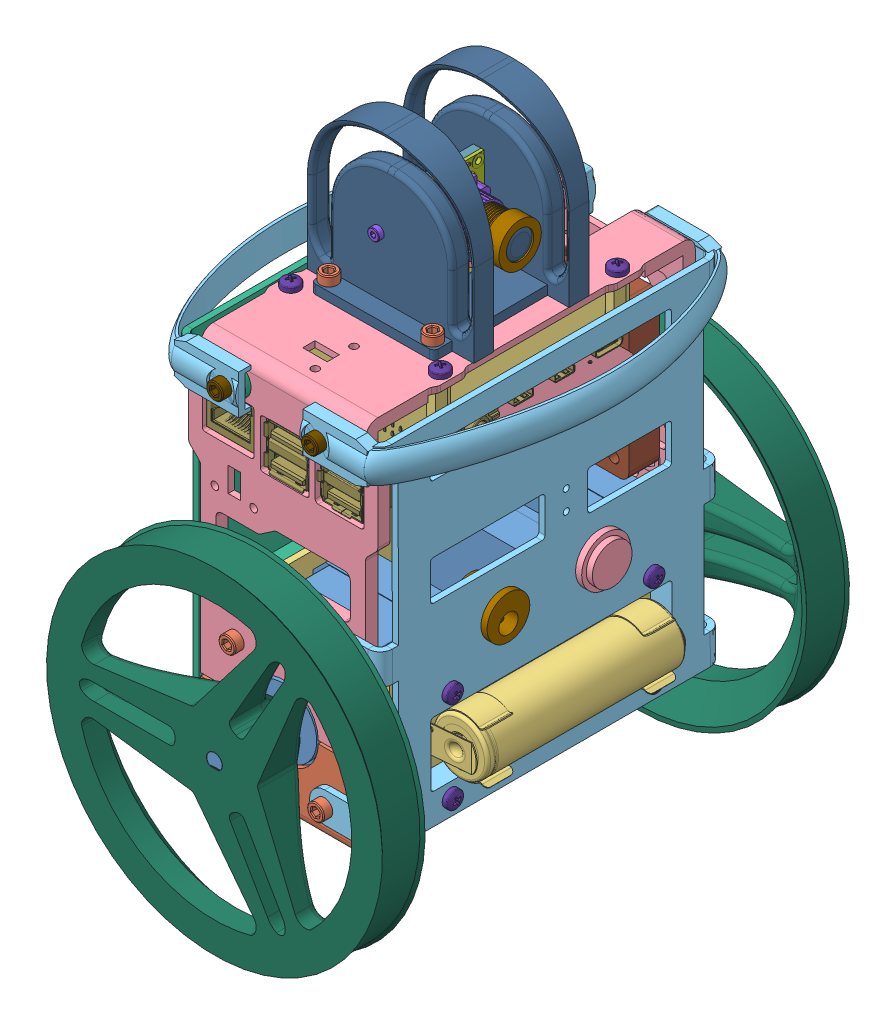
SolidWorks assembly irys5, configuration Domyślna. Lengths in mm.
Overall size (156.29 205.79 153).
91 component instances, 37 part files, 139 mates.
Components (placement in the parent):
- steppermotor-1: steppermotor [Default] at (-42.2578 -7.1789 72.25) size (42.3 42.3 64.5)
- bottomframe_rys3-1: bottomframe_rys3 [Domyślna] at (-43.1924 -29.5373 18.7182) x (0 0 -1) z (0 -1 0) size (108 54 25.86)
- steppermotor-2: steppermotor [Default] at (-42.2578 -7.1789 -31.75) x (-1 0 0) z (0 0 -1) size (42.3 42.3 64.5)
- battery_module-1: battery_module [Domyślna] at (-62.2578 -31.5373 65.25) x (0 0 -1) z (0 -1 0) size (90 40 22.7)
- topframe-1: topframe [Domyślna] at (-44.2495 88.6087 10.8694) x (0 0 -1) z (0 1 0) size (108 62 97.29)
- bumper_front-2: bumper_front [Domyślna] at (-73.7578 82.3211 20.318) x (0 0 -1) z (0 1 0) size (119.34 67.65 21.51)
- bumper_front-3: bumper_front [Domyślna] at (-10.7578 82.314 20.2704) x (0 0 -1) z (0 -1 0) size (119.34 67.65 21.51)
- imu-1: imu [Domyślna] at (-53.5985 -10.4799 25.3181) x (-0.019519 0 -0.999809) z (0 -1 0) size (10.16 22.86 2.23)
- camera_mounted-1: camera_mounted [Domyślna] at (-50.0059 110.2904 17.0046) x (-0.008727 0 -0.999962) z (0.999897 0.011413 -0.008726) size (25 24 29.88)
  - Camera Module Assem-1: Camera Module Assem [Default] at (-12.4357 -13.5775 -13.0743) size (25 24 24.98)
    - PCB 1-1: PCB 1 [Default] at (8.9736 12.851 19.5114) size (25 24 2.1)
    - Camera Block-1: Camera Block [Default] at (8.9736 15.851 20.5114) size (22 13.5 12.5)
    - Camera end-1: Camera end [Default] at (8.9736 15.851 27.3922) x (0.999924 0.012337 0) z (0 0 1) size (14 14 17.26)
    - Lenz-1: Lenz [Default] at (8.9736 15.851 43.8922) size (9 9 0.5)
    - 15 Pin Ribbon Block Assem-1: 15 Pin Ribbon Block Assem [Default] at (0.7567 20.5462 10.9417) x (1 0 0) z (0 -1 0) size (22 2.5 7)
      - 15 Pin Ribbon Block-1: 15 Pin Ribbon Block [Default] at (8.217 10.8197 14.6952) size (20 2.5 6)
      - Ribbon Clamp-1: Ribbon Clamp [Default] at (8.217 10.8197 14.6952) size (22 2.5 5)
    - 0603 Resistor-1: 0603 Resistor [Default] at (2.3268 23.572 20.4882) size (1.75 0.89 0.66)
    - 0603 Resistor-2: 0603 Resistor [Default] at (4.5768 23.572 20.4882) size (1.75 0.89 0.66)
    - 0603 Resistor-3: 0603 Resistor [Default] at (15.6203 23.5707 20.4857) size (1.75 0.89 0.66)
    - 0603 Resistor-4: 0603 Resistor [Default] at (13.3703 23.5707 20.4857) size (1.75 0.89 0.66)
  - mount-1: mount [Domyślna] at (-15.8432 -12.9016 1.4371) size (25 24 5)
- H-H_M3x12mm-1: H-H_M3x12mm [Predeterminado] at (-51.2078 -23.4959 17.65) x (0.837169 0 0.546944) z (0.546944 0 -0.837169) size (5.77 12 5)
- H-H_M3x6mm-1: H-H_M3x6mm [Predeterminado] at (-51.2078 -14.4959 17.65) x (0.837169 0 0.546944) z (0.546944 0 -0.837169) size (5.77 6 5)
- pan cross head_am-2: pan cross head_am [B18.6.7M - M3 x 0.5 x 6 Type I Cross Recessed PHMS --6N] at (-51.2078 -8.0799 17.65) x (0 -1 0) z (0 0 1) size (8.37 5.6 5.6)
- battery_module_H-2: battery_module_H [Domyślna] at (13.655 -6.0808 19.8906) x (0 0 1) z (-1 0 0) size (90 40 22.7)
  - battery_module-1: battery_module [Domyślna] at (-44.6406 -21.0981 81.7004) size (90 40 22.7)
- pan cross head_am-3: pan cross head_am [B18.6.7M - M3 x 0.5 x 6 Type I Cross Recessed PHMS --6N] at (-78.4454 -22.1789 53.25) size (8.37 5.6 5.6)
- pan cross head_am-4: pan cross head_am [B18.6.7M - M3 x 0.5 x 6 Type I Cross Recessed PHMS --6N] at (-78.4454 7.8211 53.25) size (8.37 5.6 5.6)
- pan cross head_am-5: pan cross head_am [B18.6.7M - M3 x 0.5 x 6 Type I Cross Recessed PHMS --6N] at (-78.4454 7.8211 -12.75) size (8.37 5.6 5.6)
- pan cross head_am-6: pan cross head_am [B18.6.7M - M3 x 0.5 x 6 Type I Cross Recessed PHMS --6N] at (-78.4454 -22.1789 -12.75) size (8.37 5.6 5.6)
- pan cross head_am-7: pan cross head_am [B18.6.7M - M3 x 0.5 x 6 Type I Cross Recessed PHMS --6N] at (-57.2578 -35.9373 53.25) x (0 1 0) z (0 0 1) size (8.37 5.6 5.6)
- pan cross head_am-8: pan cross head_am [B18.6.7M - M3 x 0.5 x 6 Type I Cross Recessed PHMS --6N] at (-27.2578 -35.9373 53.25) x (0 1 0) z (0 0 1) size (8.37 5.6 5.6)
- pan cross head_am-9: pan cross head_am [B18.6.7M - M3 x 0.5 x 6 Type I Cross Recessed PHMS --6N] at (-57.2578 -35.9373 -12.75) x (0 1 0) z (0 0 1) size (8.37 5.6 5.6)
- pan cross head_am-10: pan cross head_am [B18.6.7M - M3 x 0.5 x 6 Type I Cross Recessed PHMS --6N] at (-27.2578 -35.9373 -12.75) x (0 1 0) z (0 0 1) size (8.37 5.6 5.6)
- battery_module_H-3: battery_module_H [Domyślna] at (-98.1705 -8.277 19.8906) x (0 0 1) z (1 0 0) size (90 40 22.7)
  - battery_module-1: battery_module [Domyślna] at (-44.6406 -21.0981 81.7004) size (90 40 22.7)
- pan cross head_am-11: pan cross head_am [B18.6.7M - M3 x 0.5 x 6 Type I Cross Recessed PHMS --6N] at (-6.0701 -22.1789 53.25) x (-1 0 0) z (0 0.924225 0.381849) size (8.37 5.6 5.6)
- pan cross head_am-12: pan cross head_am [B18.6.7M - M3 x 0.5 x 6 Type I Cross Recessed PHMS --6N] at (-6.0701 7.8211 53.25) x (-1 0 0) z (0 0.924225 0.381849) size (8.37 5.6 5.6)
- pan cross head_am-13: pan cross head_am [B18.6.7M - M3 x 0.5 x 6 Type I Cross Recessed PHMS --6N] at (-6.0701 7.8211 -12.75) x (-1 0 0) z (0 0.924225 0.381849) size (8.37 5.6 5.6)
- pan cross head_am-14: pan cross head_am [B18.6.7M - M3 x 0.5 x 6 Type I Cross Recessed PHMS --6N] at (-6.0701 -22.1789 -12.75) x (-1 0 0) z (0 0.924225 0.381849) size (8.37 5.6 5.6)
- M3x6-1: M3x6 [Default] at (-57.7578 82.3211 -40.75) x (0 0 1) z (0.923728 0.383049 0) size (9 5.5 5.5)
- M3x6-2: M3x6 [Default] at (-26.7578 82.3211 -40.75) x (0 0 1) z (0.923728 0.383049 0) size (9 5.5 5.5)
- M3x4-1: M3x4 [Default] at (-26.7578 24.3211 -38.75) x (0 0 1) z (0.923728 0.383049 0) size (7 5.5 5.5)
- M3x4-2: M3x4 [Default] at (-57.7578 24.3211 -38.75) x (0 0 1) z (0.923728 0.383049 0) size (7 5.5 5.5)
- M3x8-1: M3x8 [Default] at (-26.7578 8.3211 -36.75) x (0 0 1) z (0.923728 0.383049 0) size (9 5.5 5.5)
- M3x8-2: M3x8 [Default] at (-57.7578 8.3211 -36.75) x (0 0 1) z (0.923728 0.383049 0) size (9 5.5 5.5)
- M3x8-3: M3x8 [Default] at (-26.7578 -22.6789 -38.75) x (0 0 1) z (-0.923728 -0.383049 0) size (9 5.5 5.5)
- M3x8-4: M3x8 [Default] at (-57.7578 -22.6789 -38.75) x (0 0 1) z (0.923728 0.383049 0) size (9 5.5 5.5)
- M3x6-3: M3x6 [Default] at (-57.7578 82.3211 81.318) x (0 0 -1) z (-0.923728 -0.383049 0) size (9 5.5 5.5)
- M3x6-4: M3x6 [Default] at (-26.7578 82.3211 81.25) x (0 0 -1) z (-0.923728 -0.383049 0) size (9 5.5 5.5)
- M3x4-3: M3x4 [Default] at (-57.7578 24.3211 79.25) x (0 0 -1) z (-0.923728 -0.383049 0) size (7 5.5 5.5)
- M3x4-4: M3x4 [Default] at (-26.7578 24.3211 79.25) x (0 0 -1) z (-0.923728 -0.383049 0) size (7 5.5 5.5)
- M3x8-5: M3x8 [Default] at (-57.7578 8.3211 77.25) x (0 0 -1) z (-0.923728 -0.383049 0) size (9 5.5 5.5)
- M3x8-6: M3x8 [Default] at (-26.7578 8.314 77.25) x (0 0 -1) z (-0.923728 -0.383049 0) size (9 5.5 5.5)
- M3x8-7: M3x8 [Default] at (-57.7578 -22.6789 79.25) x (0 0 -1) z (-0.923728 -0.383049 0) size (9 5.5 5.5)
- M3x8-8: M3x8 [Default] at (-26.7578 -22.6789 79.25) x (0 0 -1) z (-0.923728 -0.383049 0) size (9 5.5 5.5)
- H-M_M3x10x6mm-1: H-M_M3x10x6mm [Predeterminado] at (-66.7578 78.6087 47.25) size (5.77 16 5)
- H-M_M3x10x6mm-2: H-M_M3x10x6mm [Predeterminado] at (-18.2481 78.6087 47.3511) size (5.77 16 5)
- H-M_M3x10x6mm-5: H-M_M3x10x6mm [Predeterminado] at (-66.7578 78.6087 -10.7875) size (5.77 16 5)
- H-M_M3x10x6mm-6: H-M_M3x10x6mm [Predeterminado] at (-17.7578 78.6087 -10.75) size (5.77 16 5)
- pan cross head_am-15: pan cross head_am [B18.6.7M - M3 x 0.5 x 6 Type I Cross Recessed PHMS --6N] at (-66.7578 93.0087 47.25) x (0 -1 0) z (-0.546944 0 0.837169) size (8.37 5.6 5.6)
- pan cross head_am-16: pan cross head_am [B18.6.7M - M3 x 0.5 x 6 Type I Cross Recessed PHMS --6N] at (-17.7578 93.0087 -10.75) x (0 -1 0) z (-0.546944 0 0.837169) size (8.37 5.6 5.6)
- pan cross head_am-17: pan cross head_am [B18.6.7M - M3 x 0.5 x 6 Type I Cross Recessed PHMS --6N] at (-66.7578 93.0087 -10.75) x (0 -1 0) z (-0.546944 0 0.837169) size (8.37 5.6 5.6)
- pan cross head_am-18: pan cross head_am [B18.6.7M - M3 x 0.5 x 6 Type I Cross Recessed PHMS --6N] at (-17.7578 93.0087 47.25) x (0 -1 0) z (-0.546944 0 0.837169) size (8.37 5.6 5.6)
- switch_simple-1: switch_simple [Domyślna] at (-4.4625 21.3716 4.25) x (0 0 1) z (-0.999997 -0.002583 0) size (16 16 16)
- front-4: front [Domyślna] at (-10.5869 69.5154 20.4189) x (0 0 -1) z (0.002583 -0.999997 0) size (112 23.29 115)
- back-1: back [Domyślna] at (-74.0454 69.4652 19.8764) x (0 0 1) z (0 -1 0) size (112 23.29 115)
- 430250200.stp-4: 430250200.stp [Domyślna] at (-25.0029 52.3587 -6.87) x (-1 0 0) z (0 0 -1) size (5.28 14 10.85)
- 430250200.stp-5: 430250200.stp [Domyślna] at (-40.3546 52.3587 -6.985) x (-1 0 0) z (0 0 -1) size (5.28 14 10.85)
- 430250200.stp-6: 430250200.stp [Domyślna] at (-47.7558 52.3587 -6.985) x (-1 0 0) z (0 0 -1) size (5.28 14 10.85)
- 430250200.stp-7: 430250200.stp [Domyślna] at (-31.8443 52.3587 -6.985) x (-1 0 0) z (0 0 -1) size (5.28 14 10.85)
- M2 x 0.4mm Thread 10mm LONG SOCKET HEAD CAP SCREW-5: M2 x 0.4mm Thread 10mm LONG SOCKET HEAD CAP SCREW [Domyślna] at (-46.1456 112.6087 11.197) x (-0.266178 0.963921 0.002323) z (0.008727 0 0.999962) size (3.8 3.8 12.09)
- M2 x 0.4mm Thread 10mm LONG SOCKET HEAD CAP SCREW-6: M2 x 0.4mm Thread 10mm LONG SOCKET HEAD CAP SCREW [Domyślna] at (-45.9885 112.6087 29.1949) x (-0.999897 -0.011413 0.008726) z (-0.008727 0 -0.999962) size (3.8 3.8 12.09)
- M3x8-9: M3x8 [Default] at (-25.2578 96.6087 -1.75) x (0 -1 0) z (-0.923728 0 0.383049) size (9 5.5 5.5)
- M3x8-13: M3x8 [Default] at (-59.2578 96.6087 42.25) x (0 -1 0) z (-0.923728 0 0.383049) size (9 5.5 5.5)
- M3x8-14: M3x8 [Default] at (-25.2578 96.6087 42.25) x (0 -1 0) z (-0.923728 0 0.383049) size (9 5.5 5.5)
- M3x8-15: M3x8 [Default] at (-59.2578 96.6087 -1.75) x (0 -1 0) z (-0.923728 0 0.383049) size (9 5.5 5.5)
- Panel_Mount_2mm_Power_Plug_v2.step-1: Panel_Mount_2mm_Power_Plug_v2.step [Domyślna] at (-6.4559 21.3664 36.25) x (0 -0.000012 -1) z (-0.002583 0.999997 -0.000012) size (14 13.69 14)
- mount3-1: mount3 [Domyślna] at (-42.0651 90.6087 20.3975) x (-0.008727 0 -0.999962) z (0.999962 0 -0.008727) size (50 53 54.12)
- fan_simple_50x50-1: fan_simple_50x50 [Domyślna] at (-42.2578 53.8211 -24.0253) x (1 0 0) z (0 -1 0) size (50 10 50)
- Raspberry Pi 4 Model B-2: Raspberry Pi 4 Model B [Default] at (-42.2578 77.8087 28.25) x (0 0 1) z (1 0 0) size (88.99 19.91 58.4)
- rys_board_v4.1-1: rys_board_v4.1 [Domyślna] at (-94.2277 65.9587 -55.6601) x (1 0 0) z (0 -1 0) size (56.3 64 18.7)
- LD06_lidar-1: LD06_lidar [Domyślna] at (-75.5201 35.8179 20.34) x (0 0 -1) z (-0.002583 0.999997 0) size (38.59 33.3 38.59)
- Wheel_3x2_spikes-1: Wheel_3x2_spikes [Domyślna] at (-42.2578 -7.1789 96.75) x (0 0 -1) z (0 1 0) size (20 110 110)
- Wheel_3x2_spikes-2: Wheel_3x2_spikes [Domyślna] at (-42.2578 -7.1789 -56.25) x (0 0 1) z (0 1 0) size (20 110 110)
- Servo_LiDAR_hider-1: Servo_LiDAR_hider [Domyślna] at (-36.9556 74.7378 13.3028) x (0.999997 0.002583 0) z (0.002583 -0.999997 0) size (75.64 41.9 38)
  - Servo_DSM44-1: Servo_DSM44 [Default] at (-1.0294 -16.1528 31.7) size (28.2 27.4 8.5)
  - gear-1: gear [Domyślna] at (-4.9294 9.0487 31.7) x (1 0 0) z (0 1 0) size (12.97 12.88 4)
  - lidar_servo_mount-1: lidar_servo_mount [Domyślna] at (-38.6649 6.7422 39.1152) x (0 -1 0) z (0 0 1) size (38 49 38)
  - servo_holder-1: servo_holder [Domyślna] at (-1.0294 -0.0528 38.45) x (-1 0 0) z (0 0 -1) size (40.5 8 19.5)
Mates (geometry in assembly coordinates):
- Koncentryczne1: concentric aligned: cylinder of steppermotor-1 through (-26.7578 -22.6789 64.75) axis (0 0 1) radius 1.25; cylinder of bottomframe_rys3-1 through (-26.7578 -22.6789 74.25) axis (0 0 1) radius 1.6
- Koncentryczne2: concentric aligned: cylinder of steppermotor-1 through (-57.7578 -22.6789 64.75) axis (0 0 1) radius 1.25; cylinder of bottomframe_rys3-1 through (-57.7578 -22.6789 74.25) axis (0 0 1) radius 1.6
- Wspólnie1: coincident anti-aligned: plane of steppermotor-1 through (-64.2538 -29.1749 72.25) normal (0 0 1); plane of bottomframe_rys3-1 through (-42.2578 -7.6789 72.25) normal (0 0 -1)
- Koncentryczne3: concentric aligned: cylinder of bottomframe_rys3-1 through (-57.7578 -22.6789 -33.75) axis (0 0 -1) radius 1.6; cylinder of steppermotor-2 through (-57.7578 -22.6789 -24.25) axis (0 0 -1) radius 1.25
- Koncentryczne4: concentric aligned: circle of bottomframe_rys3-1; cylinder of steppermotor-2 through (-26.7578 -22.6789 -24.25) axis (0 0 -1) radius 1.25
- Wspólnie2: coincident anti-aligned: plane of bottomframe_rys3-1 through (-42.2578 -161.6789 -31.75) normal (0 0 1); plane of steppermotor-2 through (-20.2618 -29.1749 -31.75) normal (0 0 -1)
- Koncentryczne7: concentric aligned: cylinder of steppermotor-2 through (-26.7578 8.3211 -24.25) axis (0 0 -1) radius 1.25; cylinder of topframe-1 through (-26.7578 8.3211 -33.75) axis (0 0 -1) radius 1.6
- Koncentryczne8: concentric aligned: cylinder of steppermotor-1 through (-57.7578 8.3211 64.75) axis (0 0 1) radius 1.25; cylinder of topframe-1 through (-57.7578 8.3211 74.25) axis (0 0 1) radius 1.6
- Wspólnie4: coincident anti-aligned: plane of steppermotor-1 through (-64.2538 -29.1749 72.25) normal (0 0 1); plane of topframe-1 through (-71.2578 51.9927 72.25) normal (0 0 -1)
- Koncentryczne18: concentric aligned: cylinder of bottomframe_rys3-1 through (-26.7578 -22.6789 -33.75) axis (0 0 -1) radius 1.6; cylinder of steppermotor-2 through (-26.7578 -22.6789 -24.25) axis (0 0 -1) radius 1.25
- Koncentryczne55: concentric aligned: cylinder of battery_module-1 through (-51.2078 -29.4959 17.65) axis (0 1 0) radius 1.1; cylinder of imu-1 through (-51.2078 -11.4959 17.65) axis (0 1 0) radius 1.0922
- Koncentryczne56: concentric anti-aligned: cylinder of bottomframe_rys3-1 through (-27.2578 -33.5373 53.25) axis (0 -1 0) radius 1.4; cylinder of battery_module-1 through (-27.2578 -29.4959 53.25) axis (0 1 0) radius 1.6
- Koncentryczne57: concentric anti-aligned: cylinder of bottomframe_rys3-1 through (-57.2578 -33.5373 -12.75) axis (0 -1 0) radius 1.4; cylinder of battery_module-1 through (-57.2578 -29.4959 -12.75) axis (0 1 0) radius 1.6
- Wspólnie27: coincident anti-aligned: plane of bottomframe_rys3-1 through (-42.2578 -31.5373 97.25) normal (0 1 0); plane of battery_module-1 through (-62.2578 -31.5373 65.25) normal (0 -1 0)
- Wspólnie61: coincident anti-aligned: plane of topframe-1 through (-71.2578 88.6087 109.5784) normal (0 -1 0); plane of ToF_nut-5/m2_x_0_4mm_thread_hex_nut-4 through (-37.3526 88.6087 64.7673) normal (0 1 0)
- Koncentryczne104: concentric aligned: cylinder of topframe-1 through (-39.3956 90.6087 53.9072) axis (0 1 0) radius 1.25; cylinder of m2_x_0_4mm_thread_6mm_long_sock-7 through (-39.3956 92.6087 53.9072) axis (0 1 0) radius 1.9
- Wspólnie65: coincident anti-aligned: plane of topframe-1 through (-71.2578 90.6087 109.5784) normal (0 1 0); plane of m2_x_0_4mm_thread_6mm_long_sock-7 through (-39.3956 90.6087 53.9072) normal (0 -1 0)
- Wspólnie67: coincident anti-aligned: plane of topframe-1 through (-71.2578 51.9927 72.25) normal (0 0 -1); plane of ToF_nut-6/m2_x_0_4mm_thread_hex_nut-4 through (-62.7869 47.2984 72.25) normal (0 0 1)
- Wspólnie68: coincident anti-aligned: plane of topframe-1 through (-71.2578 230.6495 -31.75) normal (0 0 1); plane of ToF_nut-7/m2_x_0_4mm_thread_hex_nut-3 through (-34.075 59.7262 -31.75) normal (0 0 -1)
- Wspólnie78: coincident anti-aligned: plane of topframe-1 through (-71.2578 51.9927 74.25) normal (0 0 1); plane of m2_x_0_4mm_thread_6mm_long_sock-15 through (-64.6078 48.6087 74.25) normal (0 0 -1)
- Wspólnie79: coincident anti-aligned: plane of topframe-1 through (-71.2578 51.9927 74.25) normal (0 0 1); plane of m2_x_0_4mm_thread_6mm_long_sock-16 through (-51.9078 48.6087 74.25) normal (0 0 -1)
- Wspólnie80: coincident anti-aligned: plane of topframe-1 through (-71.2578 230.6495 -33.75) normal (0 0 -1); plane of m2_x_0_4mm_thread_6mm_long_sock-17 through (-48.6078 58.3211 -33.75) normal (0 0 1)
- Koncentryczne125: concentric aligned: cylinder of battery_module-1 through (-51.2078 -29.4959 17.65) axis (0 1 0) radius 1.1; cylinder of H-H_M3x12mm-1 through (-51.2078 -29.4959 17.65) axis (0 1 0) radius 1.5
- Wspólnie82: coincident anti-aligned: plane of battery_module-1 through (-62.2578 -29.4959 65.25) normal (0 1 0); plane of H-H_M3x12mm-1 through (-51.2078 -29.4959 17.65) normal (0 -1 0)
- Wspólnie83: coincident anti-aligned: circle of H-H_M3x12mm-1; cylinder of H-H_M3x6mm-1 through (-51.2078 -17.4959 17.65) axis (0 1 0) radius 1.5
- Wspólnie84: coincident anti-aligned: plane of H-H_M3x12mm-1 through (-51.2078 -17.4959 17.65) normal (0 1 0); plane of H-H_M3x6mm-1 through (-51.2078 -17.4959 17.65) normal (0 -1 0)
- Wspólnie85: coincident anti-aligned: plane of imu-1 through (-53.5985 -11.4959 25.3181) normal (0 -1 0); plane of H-H_M3x6mm-1 through (-51.2078 -11.4959 17.65) normal (0 1 0)
- Koncentryczne1261: concentric aligned: cylinder of imu-1 through (-51.2078 -11.4959 17.65) axis (0 1 0) radius 1.0922; cylinder of pan cross head_am-2 through (-51.2078 17.3201 17.65) axis (0 1 0) radius 2.8
- Wspólnie871: coincident anti-aligned: plane of imu-1 through (-53.5985 -10.4799 25.3181) normal (0 1 0); plane of pan cross head_am-2 through (-49.7078 -10.4799 17.65) normal (0 -1 0)
- Koncentryczne1331: concentric aligned: cylinder of bottomframe_rys3-1 through (-57.2578 -33.5373 53.25) axis (0 -1 0) radius 1.4; cylinder of pan cross head_am-7 through (-57.2578 -61.3373 53.25) axis (0 -1 0) radius 2.8
- Wspólnie931: coincident anti-aligned: plane of bottomframe_rys3-1 through (-42.2578 -33.5373 97.25) normal (0 -1 0); plane of pan cross head_am-7 through (-58.7578 -33.5373 53.25) normal (0 1 0)
- Koncentryczne1341: concentric aligned: cylinder of bottomframe_rys3-1 through (-27.2578 -33.5373 53.25) axis (0 -1 0) radius 1.4; cylinder of pan cross head_am-8 through (-27.2578 -61.3373 53.25) axis (0 -1 0) radius 2.8
- Wspólnie941: coincident anti-aligned: plane of bottomframe_rys3-1 through (-42.2578 -33.5373 97.25) normal (0 -1 0); plane of pan cross head_am-8 through (-28.7578 -33.5373 53.25) normal (0 1 0)
- Koncentryczne1351: concentric aligned: cylinder of bottomframe_rys3-1 through (-57.2578 -33.5373 -12.75) axis (0 -1 0) radius 1.4; cylinder of pan cross head_am-9 through (-57.2578 -61.3373 -12.75) axis (0 -1 0) radius 2.8
- Wspólnie951: coincident anti-aligned: plane of bottomframe_rys3-1 through (-42.2578 -33.5373 97.25) normal (0 -1 0); plane of pan cross head_am-9 through (-58.7578 -33.5373 -12.75) normal (0 1 0)
- Koncentryczne1361: concentric aligned: cylinder of bottomframe_rys3-1 through (-27.2578 -33.5373 -12.75) axis (0 -1 0) radius 1.4; cylinder of pan cross head_am-10 through (-27.2578 -61.3373 -12.75) axis (0 -1 0) radius 2.8
- Wspólnie961: coincident anti-aligned: plane of bottomframe_rys3-1 through (-42.2578 -33.5373 97.25) normal (0 -1 0); plane of pan cross head_am-10 through (-28.7578 -33.5373 -12.75) normal (0 1 0)
- Koncentryczne148: concentric aligned: cylinder of topframe-1 through (-26.7578 8.3211 -33.75) axis (0 0 -1) radius 1.6; cylinder of M3x8-1 through (-26.7578 8.3211 -125.4555) axis (0 0 -1) radius 2.75
- Wspólnie107: coincident anti-aligned: plane of topframe-1 through (-71.2578 230.6495 -33.75) normal (0 0 -1); plane of M3x8-1 through (-26.187 6.9447 -33.75) normal (0 0 1)
- Koncentryczne149: concentric aligned: cylinder of topframe-1 through (-57.7578 8.3211 -33.75) axis (0 0 -1) radius 1.6; cylinder of M3x8-2 through (-57.7578 8.3211 -125.4555) axis (0 0 -1) radius 2.75
- Wspólnie108: coincident anti-aligned: plane of topframe-1 through (-71.2578 230.6495 -33.75) normal (0 0 -1); plane of M3x8-2 through (-57.187 6.9447 -33.75) normal (0 0 1)
- Koncentryczne150: concentric aligned: cylinder of bottomframe_rys3-1 through (-57.7578 -22.6789 -33.75) axis (0 0 -1) radius 1.6; cylinder of M3x8-4 through (-57.7578 -22.6789 -127.4555) axis (0 0 -1) radius 2.75
- Koncentryczne153: concentric aligned: circle of topframe-1; cylinder of M3x6-3 through (-57.7578 82.3211 170.0235) axis (0 0 1) radius 2.75
- Koncentryczne155: concentric aligned: cylinder of topframe-1 through (-57.7578 24.3211 74.25) axis (0 0 1) radius 1.6; cylinder of M3x4-3 through (-57.7578 24.3211 167.9555) axis (0 0 1) radius 2.75
- Koncentryczne158: concentric aligned: cylinder of topframe-1 through (-26.7578 8.314 74.25) axis (0 0 1) radius 1.6; cylinder of M3x8-6 through (-26.7578 8.314 165.9555) axis (0 0 1) radius 2.75
- Koncentryczne159: concentric aligned: cylinder of topframe-1 through (-57.7578 8.3211 74.25) axis (0 0 1) radius 1.6; cylinder of M3x8-5 through (-57.7578 8.3211 165.9555) axis (0 0 1) radius 2.75
- Wspólnie115: coincident anti-aligned: plane of topframe-1 through (-71.2578 51.9927 74.25) normal (0 0 1); plane of M3x8-5 through (-57.187 6.9447 74.25) normal (0 0 -1)
- Wspólnie116: coincident anti-aligned: plane of topframe-1 through (-71.2578 51.9927 74.25) normal (0 0 1); plane of M3x8-6 through (-26.187 6.9376 74.25) normal (0 0 -1)
- Równolegle1: parallel aligned: plane of ToF_nut-7/m2_x_0_4mm_thread_hex_nut-1 through (-34.7531 56.3211 -27.53) normal (0 0 1); plane of m2_x_0_4mm_thread_6mm_long_sock-18 through (-35.9078 58.3211 -33.6076) normal (0 0 1)
- Koncentryczne1462: concentric aligned: circle of topframe-1; circle of m2_x_0_4mm_thread_6mm_long_sock-19
- Koncentryczne1463: concentric anti-aligned: circle of bumper2-1; circle of M3x6-7
- Wspólnie970: coincident anti-aligned: plane of bumper2-1 through (-6.0454 102.864 47.0753) normal (1 0 0); plane of M3x6-7 through (-6.0454 81.4447 41.6793) normal (-1 0 0)
- Koncentryczne1464: concentric anti-aligned: circle of bumper2-2; circle of M3x6-8
- Wspólnie971: coincident anti-aligned: plane of bumper2-2 through (-6.0454 102.864 3.0753) normal (1 0 0); plane of M3x6-8 through (-6.0454 81.4447 -2.3207) normal (-1 0 0)
- Koncentryczne1465: concentric aligned: circle of bumper2-1; circle of M3x6-6
- Koncentryczne1466: concentric aligned: circle of bumper2-2; circle of M3x6-5
- Koncentryczne1483: concentric aligned: circle of H-M_M3x10x6mm-1; circle of rys_PCB_rpi_simple-2
- Wspólnie978: coincident anti-aligned: plane of H-M_M3x10x6mm-1 through (-66.7578 78.6087 47.25) normal (0 -1 0); plane of rys_PCB_rpi_simple-2 through (-42.2266 78.6087 28.4747) normal (0 1 0)
- Koncentryczne1484: concentric aligned: circle of H-M_M3x10x6mm-2; circle of rys_PCB_rpi_simple-2
- Wspólnie979: coincident anti-aligned: plane of H-M_M3x10x6mm-2 through (-18.2481 78.6087 47.3511) normal (0 -1 0); plane of rys_PCB_rpi_simple-2 through (-42.2266 78.6087 28.4747) normal (0 1 0)
- Koncentryczne1485: concentric aligned: circle of H-M_M3x10x6mm-5; circle of rys_PCB_rpi_simple-2
- Wspólnie980: coincident anti-aligned: plane of H-M_M3x10x6mm-5 through (-66.7578 78.6087 -10.7875) normal (0 -1 0); plane of rys_PCB_rpi_simple-2 through (-42.2266 78.6087 28.4747) normal (0 1 0)
- Koncentryczne1486: concentric aligned: circle of H-M_M3x10x6mm-6; circle of rys_PCB_rpi_simple-2
- Wspólnie981: coincident anti-aligned: plane of H-M_M3x10x6mm-6 through (-17.7578 78.6087 -10.75) normal (0 -1 0); plane of rys_PCB_rpi_simple-2 through (-42.2266 78.6087 28.4747) normal (0 1 0)
- Koncentryczne1487: concentric anti-aligned: circle of topframe-1; circle of H-M_M3x10x6mm-1
- Wspólnie982: coincident anti-aligned: plane of topframe-1 through (-71.2578 88.6087 109.5784) normal (0 -1 0); plane of H-M_M3x10x6mm-1 through (-66.7578 88.6087 47.25) normal (0 1 0)
- Koncentryczne1490: concentric aligned: circle of topframe-1; circle of M3X6_PLASTIC-2
- Wspólnie983: coincident aligned: plane of topframe-1 through (-71.2578 90.6087 109.5784) normal (0 1 0); circle of M3X6_PLASTIC-2
- Koncentryczne1491: concentric aligned: circle of topframe-1; circle of M3X6_PLASTIC-3
- Wspólnie985: coincident aligned: plane of topframe-1 through (-71.2578 90.6087 109.5784) normal (0 1 0); circle of M3X6_PLASTIC-3
- Koncentryczne1492: concentric aligned: circle of topframe-1; circle of M3X6_PLASTIC-1
- Wspólnie986: coincident aligned: plane of topframe-1 through (-71.2578 90.6087 109.5784) normal (0 1 0); circle of M3X6_PLASTIC-1
- Koncentryczne1493: concentric aligned: circle of topframe-1; circle of M3X6_PLASTIC-4
- Wspólnie987: coincident aligned: plane of topframe-1 through (-71.2578 90.6087 109.5784) normal (0 1 0); circle of M3X6_PLASTIC-4
- Stycznie1: tangent: circle of topframe-1; circle of front-4
- Koncentryczne1502: concentric aligned: circle of topframe-1; circle of front-4
- Wspólnie1015: coincident anti-aligned: plane of topframe-1 through (-71.2578 90.6087 109.5784) normal (0 1 0); plane of m2_x_0_4mm_thread_6mm_long_sock-19 through (-39.3956 90.6087 66.6072) normal (0 -1 0)
- Równolegle8: parallel anti-aligned: plane of rys_PCB_rpi_simple-2 through (-27.3114 55.3587 -4.0403) normal (0 -1 0); plane of 430250200.stp-4 through (-26.9279 56.0087 -3.44) normal (0 1 0)
- Wspólnie1024: coincident anti-aligned: plane of rys_PCB_rpi_simple-2 through (-50.9865 55.3587 -4.0153) normal (0 -1 0); plane of 430250200.stp-6 through (-49.6808 56.0087 -3.555) normal (0 1 0)
- Wspólnie1025: coincident anti-aligned: plane of rys_PCB_rpi_simple-2 through (-43.1115 55.3587 -4.0153) normal (0 -1 0); plane of 430250200.stp-5 through (-42.2796 56.0087 -3.555) normal (0 1 0)
- Wspólnie1026: coincident anti-aligned: plane of rys_PCB_rpi_simple-2 through (-35.2115 55.3587 -4.0153) normal (0 -1 0); plane of 430250200.stp-7 through (-33.7693 56.0087 -3.555) normal (0 1 0)
- Koncentryczne1524: concentric aligned: circle of mount2-1; circle of M3x8-13
- Wspólnie1031: coincident anti-aligned: plane of mount2-1 through (-60.7578 93.6087 -3.25) normal (0 1 0); plane of M3x8-13 through (-58.687 93.6087 43.6264) normal (0 -1 0)
- Koncentryczne1525: concentric aligned: circle of mount2-1; circle of M3x8-14
- Koncentryczne1526: concentric aligned: circle of mount2-1; circle of M3x8-15
- Koncentryczne1527: concentric aligned: circle of mount2-1; circle of M3x8-9
- Wspólnie1032: coincident aligned: plane of mount2-1 through (-60.7578 93.6087 -3.25) normal (0 1 0); circle of M3x8-14
- Wspólnie1033: coincident aligned: plane of mount2-1 through (-60.7578 93.6087 -3.25) normal (0 1 0); circle of M3x8-15
- Wspólnie1034: coincident anti-aligned: plane of mount2-1 through (-60.7578 93.6087 -3.25) normal (0 1 0); plane of M3x8-9 through (-24.687 93.6087 -0.3736) normal (0 -1 0)
- Koncentryczne1531: concentric anti-aligned: circle of mount2-1; circle of M2 x 0.4mm Thread 10mm LONG SOCKET HEAD CAP SCREW-6
- Wspólnie1036: coincident anti-aligned: plane of mount2-1 through (-42.2578 133.6087 39.25) normal (0 0 1); plane of M2 x 0.4mm Thread 10mm LONG SOCKET HEAD CAP SCREW-6 through (-45.9012 112.6087 39.1945) normal (-0.008727 0 -0.999962)
- Koncentryczne1533: concentric aligned: circle of mount2-1; circle of M2 x 0.4mm Thread 10mm LONG SOCKET HEAD CAP SCREW-5
- Wspólnie1038: coincident anti-aligned: plane of mount2-1 through (-42.2578 133.6087 1.25) normal (0 0 -1); plane of M2 x 0.4mm Thread 10mm LONG SOCKET HEAD CAP SCREW-5 through (-46.2328 112.6087 1.1974) normal (0.008727 0 0.999962)
- Koncentryczne1535: concentric aligned: circle of M3x8-9; circle of mount3-1
- Wspólnie1051: coincident anti-aligned: plane of topframe-1 through (-71.2578 90.6087 109.5784) normal (0 1 0); plane of mount3-1 through (-60.7695 90.6087 -2.9402) normal (0 -1 0)
- Koncentryczne1539: concentric aligned: circle of M2 x 0.4mm Thread 10mm LONG SOCKET HEAD CAP SCREW-6; circle of mount3-1
- Koncentryczne1540: concentric anti-aligned: circle of M2 x 0.4mm Thread 10mm LONG SOCKET HEAD CAP SCREW-5; circle of mount3-1
- Wspólnie1053: coincident aligned: circle of camera_mounted-1/mount-1; circle of mount3-1
- Koncentryczne1541: concentric anti-aligned: circle of topframe-1; circle of m2_x_0_4mm_thread_6mm_long_sock-18
- Koncentryczne1542: concentric anti-aligned: circle of topframe-1; circle of m2_x_0_4mm_thread_6mm_long_sock-17
- Koncentryczne1543: concentric aligned: circle of ToF_nut-7/vl53l1x-1; circle of m2_x_0_4mm_thread_6mm_long_sock-17
- Koncentryczne1544: concentric anti-aligned: circle of topframe-1; circle of fan_simple_50x50-1
- Wspólnie1055: coincident anti-aligned: plane of rys_PCB_rpi_simple-2 through (-14.2266 78.6087 -14.0253) normal (0 0 -1); plane of fan_simple_50x50-1 through (-64.2578 31.8211 -14.0253) normal (0 0 1)
- Koncentryczne1545: concentric aligned: circle of steppermotor-1; circle of Wheel_new-1
- Wspólnie1061: coincident aligned: plane of steppermotor-1 through (-44.8633 -9.2845 96.75) normal (0 0 1); plane of Wheel_new-1 through (-28.7585 -61.3214 96.75) normal (0 0 1)
- Koncentryczne1547: concentric aligned: circle of steppermotor-2; circle of Wheel_new-2
- Wspólnie1062: coincident aligned: plane of steppermotor-2 through (-39.6522 -9.2845 -56.25) normal (0 0 -1); plane of Wheel_new-2 through (-55.757 -61.3214 -56.25) normal (0 0 -1)
- Koncentryczne1548: concentric aligned: circle of topframe-1; circle of ToF_nut-6/m2_x_0_4mm_thread_hex_nut-3
- Koncentryczne1549: concentric aligned: circle of topframe-1; circle of m2_x_0_4mm_thread_6mm_long_sock-15
- Koncentryczne1550: concentric aligned: circle of topframe-1; circle of m2_x_0_4mm_thread_6mm_long_sock-16
- Koncentryczne1554: concentric aligned: circle of topframe-1; circle of bumper_front-3
- Koncentryczne1555: concentric anti-aligned: circle of topframe-1; circle of bumper_front-2
- Koncentryczne1556: concentric anti-aligned: circle of H-M_M3x10x6mm-1; circle of Raspberry Pi 4 Model B-2
- Koncentryczne1559: concentric aligned: circle of topframe-1; circle of pan cross head_am-16
- Koncentryczne1560: concentric aligned: circle of topframe-1; circle of H-M_M3x10x6mm-6
- Koncentryczne1561: concentric aligned: circle of H-M_M3x10x6mm-6; circle of Raspberry Pi 4 Model B-2
- Wspólnie1066: coincident anti-aligned: plane of topframe-1 through (-71.2578 88.6087 109.5784) normal (0 -1 0); plane of H-M_M3x10x6mm-2 through (-18.2481 88.6087 47.3511) normal (0 1 0)
- Wspólnie1067: coincident anti-aligned: plane of H-M_M3x10x6mm-2 through (-18.2481 78.6087 47.3511) normal (0 -1 0); plane of Raspberry Pi 4 Model B-2 through (-42.2578 78.6087 28.25) normal (0 1 0)
- Wspólnie1075: coincident aligned: line of Raspberry Pi 4 Model B-2 through (-68.3478 74.5087 -5.56) axis (0 0 -1); line of rys_board_v4.1-1 through (-68.3478 74.5087 -5.2) axis (0 0 -1)
- Wspólnie1076: coincident aligned: line of Raspberry Pi 4 Model B-2 through (-68.3478 74.5087 -6.2) axis (1 0 0); line of rys_board_v4.1-1 through (-68.3478 74.5087 -6.2) axis (1 0 0)
- Wspólnie1078: coincident aligned: line of 430250200.stp-4 through (-26.2029 56.0087 -4.17) axis (1 0 0); line of rys_board_v4.1-1 through (-24.6976 56.0087 -4.17) axis (1 0 0)
- Wspólnie1079: coincident aligned: line of 430250200.stp-7 through (-30.6443 56.0087 -9.685) axis (-1 0 0); line of rys_board_v4.1-1 through (-30.0576 56.0087 -9.685) axis (-1 0 0)
- Wspólnie1080: coincident aligned: line of 430250200.stp-5 through (-39.1546 56.0087 -6.685) axis (-1 0 0); line of rys_board_v4.1-1 through (-37.9576 56.0087 -6.685) axis (-1 0 0)
- Wspólnie1081: coincident aligned: line of 430250200.stp-6 through (-46.5558 56.0087 -9.685) axis (-1 0 0); line of rys_board_v4.1-1 through (-45.8326 56.0087 -9.685) axis (-1 0 0)
- Zablokuj1: lock: unknown of topframe-1; unknown of back-1
- Wspólnie1085: coincident anti-aligned: line of back-1 through (-74.0454 42.3211 39.3764) axis (0 0 1); line of lidar_holder-1 through (-74.0454 44.5211 44.3764) axis (0 0 -1)
- Wspólnie1086: coincident anti-aligned: line of back-1 through (-74.0454 52.3211 39.3764) axis (0 -1 0); line of lidar_holder-1 through (-74.0454 44.5211 39.3764) axis (0 1 0)
- Koncentryczne1562: concentric anti-aligned: circle of lidar_holder-1; circle of k-push-1
- Wspólnie1089: coincident anti-aligned: plane of lidar_holder-1 through (-58.0454 37.0211 20.0764) normal (-1 0 0); plane of k-push-1 through (-58.0454 37.0211 20.0764) normal (1 0 0)
- Wspólnie1090: coincident anti-aligned: plane of lidar_holder-1 through (-58.0454 37.0211 20.0764) normal (-1 0 0); plane of k-push-2 through (-58.0454 39.0211 32.3764) normal (1 0 0)
- Koncentryczne1566: concentric aligned: circle of lidar_mount-1; circle of k-push-1
- Koncentryczne1567: concentric anti-aligned: circle of steppermotor-1; circle of Wheel_3x2_spikes-1
- Koncentryczne1569: concentric anti-aligned: circle of steppermotor-2; circle of Wheel_3x2_spikes-2
- Wspólnie1097: coincident aligned: plane of steppermotor-2 through (-39.6522 -9.2845 -56.25) normal (0 0 -1); plane of Wheel_3x2_spikes-2 through (11.2422 -7.1789 -56.25) normal (0 0 -1)
- Wspólnie1098: coincident anti-aligned: line of LD06_lidar-1 through (-75.5635 52.6143 1.045) axis (0.002583 -0.999997 0); line of Servo_LiDAR_hider-1/lidar_servo_mount-1 through (-75.4832 21.5229 1.045) axis (-0.002583 0.999997 0)
- Wspólnie1099: coincident aligned: line of LD06_lidar-1 through (-75.4702 16.5229 3.5435) axis (0 0 1); line of Servo_LiDAR_hider-1/lidar_servo_mount-1 through (-75.4702 16.5229 6.045) axis (0 0 1)
- Koncentryczne1570: concentric anti-aligned: circle of front-4; circle of Panel_Mount_2mm_Power_Plug_v2.step-1
- Wspólnie1109: coincident anti-aligned: plane of front-4 through (-8.62 82.361 91.25) normal (0.999997 0.002583 0); plane of Panel_Mount_2mm_Power_Plug_v2.step-1 through (-8.4625 21.3612 36.25) normal (-0.999997 -0.002583 0)
- Koncentryczne1571: concentric aligned: circle of front-4; circle of Servo_LiDAR_hider-1/servo_holder-1
